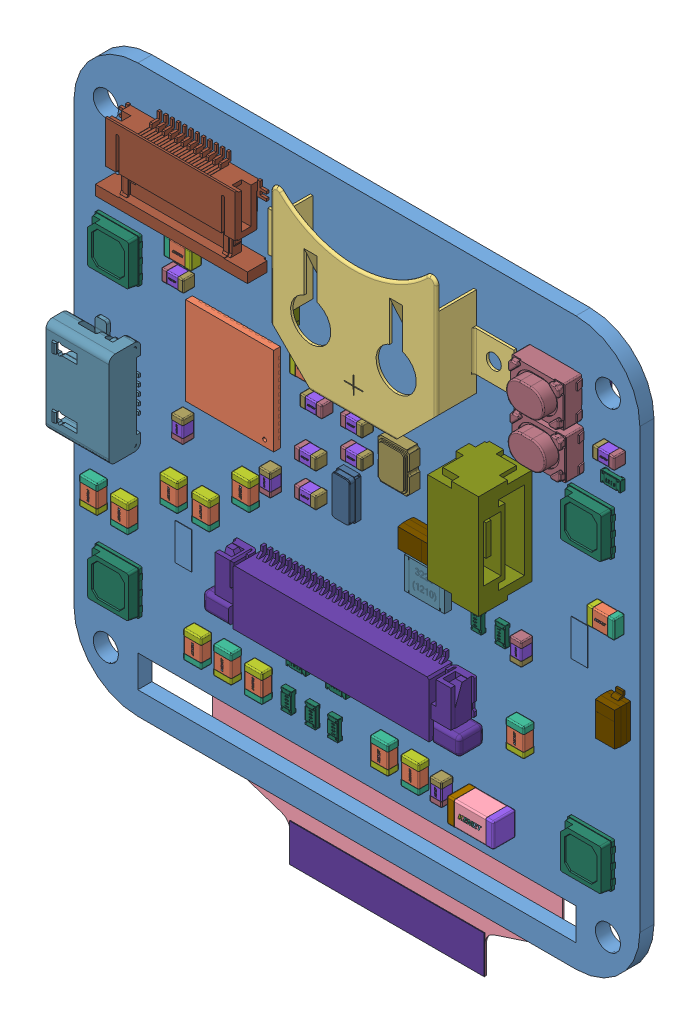
SolidWorks assembly PCB_2020-12-27_16-28-50_2021-02-20_20-59-34, configuration 默认. Lengths in mm.
Overall size (45.01 51.47 7.58).
307 component instances, 72 part files, 0 mates.
Components (placement in the parent):
- PCB_2020-12-27_16-28-50_2021-02-20_20-59-34.step-1: PCB_2020-12-27_16-28-50_2021-02-20_20-59-34.step [默认] at origin size (45.01 51.47 7.58)
  - Board.step-1: Board.step [默认] at origin size (45.01 45.01 1.12)
    - Open CASCADE STEP translator 6.8 3.1.1.step-1: Open CASCADE STEP translator 6.8 3.1.1.step [默认] at (0 0 -1.1227) size (45.01 45.01 1.12)
  - C34.step-1: C34.step [默认] at origin size (2.2 1.45 0.88)
    - c0805c101k5gactu.step-1: c0805c101k5gactu.step [默认] at (159.963 120.323 -10.6426) x (1 0 0) z (0 -1 0) size (2.2 0.88 1.45)
      - Open CASCADE STEP translator 6.8 3.2.1.1.step-1: Open CASCADE STEP translator 6.8 3.2.1.1.step [默认] at origin size (2 0.86 1.43)
      - Open CASCADE STEP translator 6.8 3.2.1.2.step-1: Open CASCADE STEP translator 6.8 3.2.1.2.step [默认] at origin size (0.34 0 0.18)
      - Open CASCADE STEP translator 6.8 3.2.1.3.step-1: Open CASCADE STEP translator 6.8 3.2.1.3.step [默认] at origin size (0.41 0 0.18)
      - Open CASCADE STEP translator 6.8 3.2.1.4.step-1: Open CASCADE STEP translator 6.8 3.2.1.4.step [默认] at origin size (0.21 0 0.18)
      - Open CASCADE STEP translator 6.8 3.2.1.5.step-1: Open CASCADE STEP translator 6.8 3.2.1.5.step [默认] at origin size (0.5 0.88 1.45)
      - Open CASCADE STEP translator 6.8 3.2.1.6.step-1: Open CASCADE STEP translator 6.8 3.2.1.6.step [默认] at origin size (0.5 0.88 1.45)
  - C14.step-1: C14.step [默认] at origin size (1.45 2.2 0.88)
    - c0805c101k5gactu.step-1: c0805c101k5gactu.step [默认] at (101.7169 -30.907 -10.6426) x (0 -1 0) z (-1 0 0) size (2.2 0.88 1.45)
      - Open CASCADE STEP translator 6.8 3.2.1.1.step-1: Open CASCADE STEP translator 6.8 3.2.1.1.step [默认] at origin size (2 0.86 1.43)
      - Open CASCADE STEP translator 6.8 3.2.1.2.step-1: Open CASCADE STEP translator 6.8 3.2.1.2.step [默认] at origin size (0.34 0 0.18)
      - Open CASCADE STEP translator 6.8 3.2.1.3.step-1: Open CASCADE STEP translator 6.8 3.2.1.3.step [默认] at origin size (0.41 0 0.18)
      - Open CASCADE STEP translator 6.8 3.2.1.4.step-1: Open CASCADE STEP translator 6.8 3.2.1.4.step [默认] at origin size (0.21 0 0.18)
      - Open CASCADE STEP translator 6.8 3.2.1.5.step-1: Open CASCADE STEP translator 6.8 3.2.1.5.step [默认] at origin size (0.5 0.88 1.45)
      - Open CASCADE STEP translator 6.8 3.2.1.6.step-1: Open CASCADE STEP translator 6.8 3.2.1.6.step [默认] at origin size (0.5 0.88 1.45)
  - C13.step-1: C13.step [默认] at origin size (0.95 1.77 0.95)
    - c0603x104k3ractu.step-1: c0603x104k3ractu.step [默认] at (16.3625 164.212 -10.6426) x (0 1 0) z (1 0 0) size (1.77 0.95 0.95)
      - Open CASCADE STEP translator 6.8 3.4.1.1.step-1: Open CASCADE STEP translator 6.8 3.4.1.1.step [默认] at origin size (1.57 0.93 0.93)
      - Open CASCADE STEP translator 6.8 3.4.1.2.step-1: Open CASCADE STEP translator 6.8 3.4.1.2.step [默认] at origin size (0.24 0 0.13)
      - Open CASCADE STEP translator 6.8 3.4.1.3.step-1: Open CASCADE STEP translator 6.8 3.4.1.3.step [默认] at origin size (0.29 0 0.13)
      - Open CASCADE STEP translator 6.8 3.4.1.4.step-1: Open CASCADE STEP translator 6.8 3.4.1.4.step [默认] at origin size (0.15 0 0.13)
      - Open CASCADE STEP translator 6.8 3.4.1.5.step-1: Open CASCADE STEP translator 6.8 3.4.1.5.step [默认] at origin size (0.45 0.95 0.95)
      - Open CASCADE STEP translator 6.8 3.4.1.6.step-1: Open CASCADE STEP translator 6.8 3.4.1.6.step [默认] at origin size (0.45 0.95 0.95)
  - C12.step-1: C12.step [默认] at origin size (0.95 1.77 0.95)
    - c0603x104k3ractu.step-1: c0603x104k3ractu.step [默认] at (9.3976 164.422 -10.6426) x (0 1 0) z (1 0 0) size (1.77 0.95 0.95)
      - Open CASCADE STEP translator 6.8 3.4.1.1.step-1: Open CASCADE STEP translator 6.8 3.4.1.1.step [默认] at origin size (1.57 0.93 0.93)
      - Open CASCADE STEP translator 6.8 3.4.1.2.step-1: Open CASCADE STEP translator 6.8 3.4.1.2.step [默认] at origin size (0.24 0 0.13)
      - Open CASCADE STEP translator 6.8 3.4.1.3.step-1: Open CASCADE STEP translator 6.8 3.4.1.3.step [默认] at origin size (0.29 0 0.13)
      - Open CASCADE STEP translator 6.8 3.4.1.4.step-1: Open CASCADE STEP translator 6.8 3.4.1.4.step [默认] at origin size (0.15 0 0.13)
      - Open CASCADE STEP translator 6.8 3.4.1.5.step-1: Open CASCADE STEP translator 6.8 3.4.1.5.step [默认] at origin size (0.45 0.95 0.95)
      - Open CASCADE STEP translator 6.8 3.4.1.6.step-1: Open CASCADE STEP translator 6.8 3.4.1.6.step [默认] at origin size (0.45 0.95 0.95)
  - USB2.step-1: USB2.step [默认] at origin size (5 7.8 2.7)
    - User_Library-micro_usb_SMD_RGB8421504.step-1: User_Library-micro_usb_SMD_RGB8421504.step [默认] at (44.3599 67.8551 1.27) x (0 -1 0) z (-1 0 0) size (7.8 2.7 5)
  - R7.step-1: R7.step [默认] at origin size (1.6 0.8 0.42)
    - User_Library-Res-0603.step-1: User_Library-Res-0603.step [默认] at (87.122 80.8989 0) x (-1 0 0) z (0 1 0) size (1.6 0.42 0.8)
  - L2.step-1: L2.step [默认] at origin size (0.86 1.6 0.51)
    - CircuitWorks-RESISTOR_0603.step-1: CircuitWorks-RESISTOR_0603.step [默认] at (61.595 79.7559 0) x (0 -1 0) z (-1 0 0) size (1.6 0.51 0.86)
  - P2.step-1: P2.step [默认] at origin size (20.43 5.11 2.05)
    - 3-1734839-0_RGB8421504.step-1: 3-1734839-0_RGB8421504.step [默认] at (66.548 57.4041 1.0414) x (1 0 0) z (0 -1 0) size (20.43 2.05 5.11)
  - D4.step-1: D4.step [默认] at origin size (3.7 1.6 1.27)
    - CircuitWorks-SOD123.step-1: CircuitWorks-SOD123.step [默认] at (72.4968 69.5129 0.0508) x (1 0 0) z (0 -1 0) size (3.7 1.27 1.6)
  - D5.step-1: D5.step [默认] at origin size (1.6 3.7 1.27)
    - CircuitWorks-SOD123.step-1: CircuitWorks-SOD123.step [默认] at (87.6301 64.8969 0.0508) x (0 1 0) z (1 0 0) size (3.7 1.27 1.6)
  - C21.step-1: C21.step [默认] at origin size (1.45 2.2 0.88)
    - c0805c101k5gactu.step-1: c0805c101k5gactu.step [默认] at (98.5419 -33.828 -10.6426) x (0 -1 0) z (-1 0 0) size (2.2 0.88 1.45)
      - Open CASCADE STEP translator 6.8 3.2.1.1.step-1: Open CASCADE STEP translator 6.8 3.2.1.1.step [默认] at origin size (2 0.86 1.43)
      - Open CASCADE STEP translator 6.8 3.2.1.2.step-1: Open CASCADE STEP translator 6.8 3.2.1.2.step [默认] at origin size (0.34 0 0.18)
      - Open CASCADE STEP translator 6.8 3.2.1.3.step-1: Open CASCADE STEP translator 6.8 3.2.1.3.step [默认] at origin size (0.41 0 0.18)
      - Open CASCADE STEP translator 6.8 3.2.1.4.step-1: Open CASCADE STEP translator 6.8 3.2.1.4.step [默认] at origin size (0.21 0 0.18)
      - Open CASCADE STEP translator 6.8 3.2.1.5.step-1: Open CASCADE STEP translator 6.8 3.2.1.5.step [默认] at origin size (0.5 0.88 1.45)
      - Open CASCADE STEP translator 6.8 3.2.1.6.step-1: Open CASCADE STEP translator 6.8 3.2.1.6.step [默认] at origin size (0.5 0.88 1.45)
  - C24.step-1: C24.step [默认] at origin size (1.45 2.2 0.88)
    - c0805c101k5gactu.step-1: c0805c101k5gactu.step [默认] at (2.51 156.471 -10.6426) x (0 1 0) z (1 0 0) size (2.2 0.88 1.45)
      - Open CASCADE STEP translator 6.8 3.2.1.1.step-1: Open CASCADE STEP translator 6.8 3.2.1.1.step [默认] at origin size (2 0.86 1.43)
      - Open CASCADE STEP translator 6.8 3.2.1.2.step-1: Open CASCADE STEP translator 6.8 3.2.1.2.step [默认] at origin size (0.34 0 0.18)
      - Open CASCADE STEP translator 6.8 3.2.1.3.step-1: Open CASCADE STEP translator 6.8 3.2.1.3.step [默认] at origin size (0.41 0 0.18)
      - Open CASCADE STEP translator 6.8 3.2.1.4.step-1: Open CASCADE STEP translator 6.8 3.2.1.4.step [默认] at origin size (0.21 0 0.18)
      - Open CASCADE STEP translator 6.8 3.2.1.5.step-1: Open CASCADE STEP translator 6.8 3.2.1.5.step [默认] at origin size (0.5 0.88 1.45)
      - Open CASCADE STEP translator 6.8 3.2.1.6.step-1: Open CASCADE STEP translator 6.8 3.2.1.6.step [默认] at origin size (0.5 0.88 1.45)
  - U7.step-1: U7.step [默认] at origin size (2.5 3 1.1)
    - CircuitWorks-SOT-23-5.step-1: CircuitWorks-SOT-23-5.step [默认] at (84.308 68.2431 -0.5131) x (0 1 0) z (1 0 0) size (3 1.1 2.5)
  - U5.step-1: U5.step [默认] at origin size (7 7 0.55)
    - User_Library-UFQFPN48.step-1: User_Library-UFQFPN48.step [默认] at (57.0029 73.1959 0) x (-1 0 0) z (0 0 1) size (7 7 0.55)
  - R13.step-1: R13.step [默认] at origin size (0.8 1.6 0.42)
    - User_Library-Res-0603.step-1: User_Library-Res-0603.step [默认] at (78.3388 65.957 0) x (0 1 0) z (1 0 0) size (1.6 0.42 0.8)
  - U4.step-1: U4.step [默认] at origin size (19.57 12.72 3.54)
    - User_Library-BK-885-TR.step-1: User_Library-BK-885-TR.step [默认] at (69.4691 84.328 0) x (1 0 0) z (0 -1 0) size (19.57 3.54 12.72)
  - U3.step-1: U3.step [默认] at origin size (0.8 1.6 0.42)
    - User_Library-Res-0603.step-1: User_Library-Res-0603.step [默认] at (61.3211 52.876 0) x (0 -1 0) z (-1 0 0) size (1.6 0.42 0.8)
  - C27.step-1: C27.step [默认] at origin size (0.95 1.77 0.95)
    - c0603x104k3ractu.step-1: c0603x104k3ractu.step [默认] at (123.9324 -30.647 -10.6426) x (0 -1 0) z (-1 0 0) size (1.77 0.95 0.95)
      - Open CASCADE STEP translator 6.8 3.4.1.1.step-1: Open CASCADE STEP translator 6.8 3.4.1.1.step [默认] at origin size (1.57 0.93 0.93)
      - Open CASCADE STEP translator 6.8 3.4.1.2.step-1: Open CASCADE STEP translator 6.8 3.4.1.2.step [默认] at origin size (0.24 0 0.13)
      - Open CASCADE STEP translator 6.8 3.4.1.3.step-1: Open CASCADE STEP translator 6.8 3.4.1.3.step [默认] at origin size (0.29 0 0.13)
      - Open CASCADE STEP translator 6.8 3.4.1.4.step-1: Open CASCADE STEP translator 6.8 3.4.1.4.step [默认] at origin size (0.15 0 0.13)
      - Open CASCADE STEP translator 6.8 3.4.1.5.step-1: Open CASCADE STEP translator 6.8 3.4.1.5.step [默认] at origin size (0.45 0.95 0.95)
      - Open CASCADE STEP translator 6.8 3.4.1.6.step-1: Open CASCADE STEP translator 6.8 3.4.1.6.step [默认] at origin size (0.45 0.95 0.95)
  - C20.step-1: C20.step [默认] at origin size (3.7 1.95 1.8)
    - c1206x223j2gacauto.step-1: c1206x223j2gacauto.step [默认] at (174.9253 96.5054 -10.6426) x (1 0 0) z (0 -1 0) size (3.7 1.8 1.95)
      - Open CASCADE STEP translator 6.8 3.20.1.1.step-1: Open CASCADE STEP translator 6.8 3.20.1.1.step [默认] at origin size (3.5 1.78 1.93)
      - Open CASCADE STEP translator 6.8 3.20.1.2.step-1: Open CASCADE STEP translator 6.8 3.20.1.2.step [默认] at origin size (0.7 0 0.37)
      - Open CASCADE STEP translator 6.8 3.20.1.3.step-1: Open CASCADE STEP translator 6.8 3.20.1.3.step [默认] at origin size (0.85 0 0.37)
      - Open CASCADE STEP translator 6.8 3.20.1.4.step-1: Open CASCADE STEP translator 6.8 3.20.1.4.step [默认] at origin size (0.44 0 0.37)
      - Open CASCADE STEP translator 6.8 3.20.1.5.step-1: Open CASCADE STEP translator 6.8 3.20.1.5.step [默认] at origin size (0.6 1.8 1.95)
      - Open CASCADE STEP translator 6.8 3.20.1.6.step-1: Open CASCADE STEP translator 6.8 3.20.1.6.step [默认] at origin size (0.6 1.8 1.95)
  - X3.step-1: X3.step [默认] at origin size (1.5 3.2 0.91)
    - crystal_rtf3215.step-1: crystal_rtf3215.step [默认] at (66.167 69.4691 0) x (0 1 0) z (1 0 0) size (3.2 0.91 1.5)
  - C28.step-1: C28.step [默认] at origin size (1.45 2.2 0.88)
    - c0805c101k5gactu.step-1: c0805c101k5gactu.step [默认] at (25.644 150.077 -10.6426) x (0 1 0) z (1 0 0) size (2.2 0.88 1.45)
      - Open CASCADE STEP translator 6.8 3.2.1.1.step-1: Open CASCADE STEP translator 6.8 3.2.1.1.step [默认] at origin size (2 0.86 1.43)
      - Open CASCADE STEP translator 6.8 3.2.1.2.step-1: Open CASCADE STEP translator 6.8 3.2.1.2.step [默认] at origin size (0.34 0 0.18)
      - Open CASCADE STEP translator 6.8 3.2.1.3.step-1: Open CASCADE STEP translator 6.8 3.2.1.3.step [默认] at origin size (0.41 0 0.18)
      - Open CASCADE STEP translator 6.8 3.2.1.4.step-1: Open CASCADE STEP translator 6.8 3.2.1.4.step [默认] at origin size (0.21 0 0.18)
      - Open CASCADE STEP translator 6.8 3.2.1.5.step-1: Open CASCADE STEP translator 6.8 3.2.1.5.step [默认] at origin size (0.5 0.88 1.45)
      - Open CASCADE STEP translator 6.8 3.2.1.6.step-1: Open CASCADE STEP translator 6.8 3.2.1.6.step [默认] at origin size (0.5 0.88 1.45)
  - C29.step-1: C29.step [默认] at origin size (1.45 2.2 0.88)
    - c0805c101k5gactu.step-1: c0805c101k5gactu.step [默认] at (102.7329 -43.6071 -10.6426) x (0 -1 0) z (-1 0 0) size (2.2 0.88 1.45)
      - Open CASCADE STEP translator 6.8 3.2.1.1.step-1: Open CASCADE STEP translator 6.8 3.2.1.1.step [默认] at origin size (2 0.86 1.43)
      - Open CASCADE STEP translator 6.8 3.2.1.2.step-1: Open CASCADE STEP translator 6.8 3.2.1.2.step [默认] at origin size (0.34 0 0.18)
      - Open CASCADE STEP translator 6.8 3.2.1.3.step-1: Open CASCADE STEP translator 6.8 3.2.1.3.step [默认] at origin size (0.41 0 0.18)
      - Open CASCADE STEP translator 6.8 3.2.1.4.step-1: Open CASCADE STEP translator 6.8 3.2.1.4.step [默认] at origin size (0.21 0 0.18)
      - Open CASCADE STEP translator 6.8 3.2.1.5.step-1: Open CASCADE STEP translator 6.8 3.2.1.5.step [默认] at origin size (0.5 0.88 1.45)
      - Open CASCADE STEP translator 6.8 3.2.1.6.step-1: Open CASCADE STEP translator 6.8 3.2.1.6.step [默认] at origin size (0.5 0.88 1.45)
  - C30.step-1: C30.step [默认] at origin size (1.45 2.2 0.88)
    - c0805c101k5gactu.step-1: c0805c101k5gactu.step [默认] at (97.9069 -43.6071 -10.6426) x (0 -1 0) z (-1 0 0) size (2.2 0.88 1.45)
      - Open CASCADE STEP translator 6.8 3.2.1.1.step-1: Open CASCADE STEP translator 6.8 3.2.1.1.step [默认] at origin size (2 0.86 1.43)
      - Open CASCADE STEP translator 6.8 3.2.1.2.step-1: Open CASCADE STEP translator 6.8 3.2.1.2.step [默认] at origin size (0.34 0 0.18)
      - Open CASCADE STEP translator 6.8 3.2.1.3.step-1: Open CASCADE STEP translator 6.8 3.2.1.3.step [默认] at origin size (0.41 0 0.18)
      - Open CASCADE STEP translator 6.8 3.2.1.4.step-1: Open CASCADE STEP translator 6.8 3.2.1.4.step [默认] at origin size (0.21 0 0.18)
      - Open CASCADE STEP translator 6.8 3.2.1.5.step-1: Open CASCADE STEP translator 6.8 3.2.1.5.step [默认] at origin size (0.5 0.88 1.45)
      - Open CASCADE STEP translator 6.8 3.2.1.6.step-1: Open CASCADE STEP translator 6.8 3.2.1.6.step [默认] at origin size (0.5 0.88 1.45)
  - U6.step-1: U6.step [默认] at origin size (2.5 3 1.1)
    - CircuitWorks-SOT-23-5.step-1: CircuitWorks-SOT-23-5.step [默认] at (52.8119 59.0989 -0.5131) x (0 -1 0) z (-1 0 0) size (3 1.1 2.5)
  - FPC1.step-1: FPC1.step [默认] at origin size (12.1 6.6 2)
    - 52746-1290_RGB10066329.step-1: 52746-1290_RGB10066329.step [默认] at (53.7211 87.5031 0) x (1 0 0) z (0 -1 0) size (12.1 2 6.6)
  - C18.step-1: C18.step [默认] at origin size (0.95 1.77 0.95)
    - c0603x104k3ractu.step-1: c0603x104k3ractu.step [默认] at (29.9716 149.69 -10.6426) x (0 1 0) z (1 0 0) size (1.77 0.95 0.95)
      - Open CASCADE STEP translator 6.8 3.4.1.1.step-1: Open CASCADE STEP translator 6.8 3.4.1.1.step [默认] at origin size (1.57 0.93 0.93)
      - Open CASCADE STEP translator 6.8 3.4.1.2.step-1: Open CASCADE STEP translator 6.8 3.4.1.2.step [默认] at origin size (0.24 0 0.13)
      - Open CASCADE STEP translator 6.8 3.4.1.3.step-1: Open CASCADE STEP translator 6.8 3.4.1.3.step [默认] at origin size (0.29 0 0.13)
      - Open CASCADE STEP translator 6.8 3.4.1.4.step-1: Open CASCADE STEP translator 6.8 3.4.1.4.step [默认] at origin size (0.15 0 0.13)
      - Open CASCADE STEP translator 6.8 3.4.1.5.step-1: Open CASCADE STEP translator 6.8 3.4.1.5.step [默认] at origin size (0.45 0.95 0.95)
      - Open CASCADE STEP translator 6.8 3.4.1.6.step-1: Open CASCADE STEP translator 6.8 3.4.1.6.step [默认] at origin size (0.45 0.95 0.95)
  - X1.step-1: X1.step [默认] at origin size (2.5 3.2 1.05)
    - User_Library-SMD-3225_4P.step-1: User_Library-SMD-3225_4P.step [默认] at (70.338 73.8309 0) x (0 -1 0) z (0 0 1) size (3.2 2.5 1.05)
  - C26.step-1: C26.step [默认] at origin size (2.2 1.45 0.88)
    - c0805c101k5gactu.step-1: c0805c101k5gactu.step [默认] at (183.605 114.818 -10.6426) x (1 0 0) z (0 -1 0) size (2.2 0.88 1.45)
      - Open CASCADE STEP translator 6.8 3.2.1.1.step-1: Open CASCADE STEP translator 6.8 3.2.1.1.step [默认] at origin size (2 0.86 1.43)
      - Open CASCADE STEP translator 6.8 3.2.1.2.step-1: Open CASCADE STEP translator 6.8 3.2.1.2.step [默认] at origin size (0.34 0 0.18)
      - Open CASCADE STEP translator 6.8 3.2.1.3.step-1: Open CASCADE STEP translator 6.8 3.2.1.3.step [默认] at origin size (0.41 0 0.18)
      - Open CASCADE STEP translator 6.8 3.2.1.4.step-1: Open CASCADE STEP translator 6.8 3.2.1.4.step [默认] at origin size (0.21 0 0.18)
      - Open CASCADE STEP translator 6.8 3.2.1.5.step-1: Open CASCADE STEP translator 6.8 3.2.1.5.step [默认] at origin size (0.5 0.88 1.45)
      - Open CASCADE STEP translator 6.8 3.2.1.6.step-1: Open CASCADE STEP translator 6.8 3.2.1.6.step [默认] at origin size (0.5 0.88 1.45)
  - C25.step-1: C25.step [默认] at origin size (1.45 2.2 0.88)
    - c0805c101k5gactu.step-1: c0805c101k5gactu.step [默认] at (36.439 156.681 -10.6426) x (0 1 0) z (1 0 0) size (2.2 0.88 1.45)
      - Open CASCADE STEP translator 6.8 3.2.1.1.step-1: Open CASCADE STEP translator 6.8 3.2.1.1.step [默认] at origin size (2 0.86 1.43)
      - Open CASCADE STEP translator 6.8 3.2.1.2.step-1: Open CASCADE STEP translator 6.8 3.2.1.2.step [默认] at origin size (0.34 0 0.18)
      - Open CASCADE STEP translator 6.8 3.2.1.3.step-1: Open CASCADE STEP translator 6.8 3.2.1.3.step [默认] at origin size (0.41 0 0.18)
      - Open CASCADE STEP translator 6.8 3.2.1.4.step-1: Open CASCADE STEP translator 6.8 3.2.1.4.step [默认] at origin size (0.21 0 0.18)
      - Open CASCADE STEP translator 6.8 3.2.1.5.step-1: Open CASCADE STEP translator 6.8 3.2.1.5.step [默认] at origin size (0.5 0.88 1.45)
      - Open CASCADE STEP translator 6.8 3.2.1.6.step-1: Open CASCADE STEP translator 6.8 3.2.1.6.step [默认] at origin size (0.5 0.88 1.45)
  - R17.step-1: R17.step [默认] at origin size (1.6 0.8 0.42)
    - User_Library-Res-0603.step-1: User_Library-Res-0603.step [默认] at (65.278 55.7531 0) x (1 0 0) z (0 -1 0) size (1.6 0.42 0.8)
  - R12.step-1: R12.step [默认] at origin size (0.8 1.6 0.42)
    - User_Library-Res-0603.step-1: User_Library-Res-0603.step [默认] at (63.2461 52.832 0) x (0 -1 0) z (-1 0 0) size (1.6 0.42 0.8)
  - R16.step-1: R16.step [默认] at origin size (1.6 0.8 0.42)
    - User_Library-Res-0603.step-1: User_Library-Res-0603.step [默认] at (62.103 55.7529 0) x (-1 0 0) z (0 1 0) size (1.6 0.42 0.8)
  - R15.step-1: R15.step [默认] at origin size (0.8 1.6 0.42)
    - User_Library-Res-0603.step-1: User_Library-Res-0603.step [默认] at (65.0241 52.832 0) x (0 -1 0) z (-1 0 0) size (1.6 0.42 0.8)
  - SW2.step-1: SW2.step [默认] at origin size (4.6 3.2 2.5)
    - skrpace010_RGB10066329.step-1: skrpace010_RGB10066329.step [默认] at (82.5499 81.661 0) x (-1 0 0) z (0 1 0) size (4.6 2.5 3.2)
  - SW1.step-1: SW1.step [默认] at origin size (4.6 3.2 2.5)
    - skrpace010_RGB10066329.step-1: skrpace010_RGB10066329.step [默认] at (82.4231 85.217 0) x (1 0 0) z (0 -1 0) size (4.6 2.5 3.2)
  - C17.step-1: C17.step [默认] at origin size (1.77 0.95 0.95)
    - c0603x104k3ractu.step-1: c0603x104k3ractu.step [默认] at (159.977 114.6814 -10.6426) x (1 0 0) z (0 -1 0) size (1.77 0.95 0.95)
      - Open CASCADE STEP translator 6.8 3.4.1.1.step-1: Open CASCADE STEP translator 6.8 3.4.1.1.step [默认] at origin size (1.57 0.93 0.93)
      - Open CASCADE STEP translator 6.8 3.4.1.2.step-1: Open CASCADE STEP translator 6.8 3.4.1.2.step [默认] at origin size (0.24 0 0.13)
      - Open CASCADE STEP translator 6.8 3.4.1.3.step-1: Open CASCADE STEP translator 6.8 3.4.1.3.step [默认] at origin size (0.29 0 0.13)
      - Open CASCADE STEP translator 6.8 3.4.1.4.step-1: Open CASCADE STEP translator 6.8 3.4.1.4.step [默认] at origin size (0.15 0 0.13)
      - Open CASCADE STEP translator 6.8 3.4.1.5.step-1: Open CASCADE STEP translator 6.8 3.4.1.5.step [默认] at origin size (0.45 0.95 0.95)
      - Open CASCADE STEP translator 6.8 3.4.1.6.step-1: Open CASCADE STEP translator 6.8 3.4.1.6.step [默认] at origin size (0.45 0.95 0.95)
  - C19.step-1: C19.step [默认] at origin size (1.77 0.95 0.95)
    - c0603x104k3ractu.step-1: c0603x104k3ractu.step [默认] at (159.977 112.0144 -10.6426) x (1 0 0) z (0 -1 0) size (1.77 0.95 0.95)
      - Open CASCADE STEP translator 6.8 3.4.1.1.step-1: Open CASCADE STEP translator 6.8 3.4.1.1.step [默认] at origin size (1.57 0.93 0.93)
      - Open CASCADE STEP translator 6.8 3.4.1.2.step-1: Open CASCADE STEP translator 6.8 3.4.1.2.step [默认] at origin size (0.24 0 0.13)
      - Open CASCADE STEP translator 6.8 3.4.1.3.step-1: Open CASCADE STEP translator 6.8 3.4.1.3.step [默认] at origin size (0.29 0 0.13)
      - Open CASCADE STEP translator 6.8 3.4.1.4.step-1: Open CASCADE STEP translator 6.8 3.4.1.4.step [默认] at origin size (0.15 0 0.13)
      - Open CASCADE STEP translator 6.8 3.4.1.5.step-1: Open CASCADE STEP translator 6.8 3.4.1.5.step [默认] at origin size (0.45 0.95 0.95)
      - Open CASCADE STEP translator 6.8 3.4.1.6.step-1: Open CASCADE STEP translator 6.8 3.4.1.6.step [默认] at origin size (0.45 0.95 0.95)
  - C16.step-1: C16.step [默认] at origin size (1.77 0.95 0.95)
    - c0603x104k3ractu.step-1: c0603x104k3ractu.step [默认] at (163.64 118.7894 -10.6426) x (1 0 0) z (0 -1 0) size (1.77 0.95 0.95)
      - Open CASCADE STEP translator 6.8 3.4.1.1.step-1: Open CASCADE STEP translator 6.8 3.4.1.1.step [默认] at origin size (1.57 0.93 0.93)
      - Open CASCADE STEP translator 6.8 3.4.1.2.step-1: Open CASCADE STEP translator 6.8 3.4.1.2.step [默认] at origin size (0.24 0 0.13)
      - Open CASCADE STEP translator 6.8 3.4.1.3.step-1: Open CASCADE STEP translator 6.8 3.4.1.3.step [默认] at origin size (0.29 0 0.13)
      - Open CASCADE STEP translator 6.8 3.4.1.4.step-1: Open CASCADE STEP translator 6.8 3.4.1.4.step [默认] at origin size (0.15 0 0.13)
      - Open CASCADE STEP translator 6.8 3.4.1.5.step-1: Open CASCADE STEP translator 6.8 3.4.1.5.step [默认] at origin size (0.45 0.95 0.95)
      - Open CASCADE STEP translator 6.8 3.4.1.6.step-1: Open CASCADE STEP translator 6.8 3.4.1.6.step [默认] at origin size (0.45 0.95 0.95)
  - C15.step-1: C15.step [默认] at origin size (1.77 0.95 0.95)
    - c0603x104k3ractu.step-1: c0603x104k3ractu.step [默认] at (163.64 116.5034 -10.6426) x (1 0 0) z (0 -1 0) size (1.77 0.95 0.95)
      - Open CASCADE STEP translator 6.8 3.4.1.1.step-1: Open CASCADE STEP translator 6.8 3.4.1.1.step [默认] at origin size (1.57 0.93 0.93)
      - Open CASCADE STEP translator 6.8 3.4.1.2.step-1: Open CASCADE STEP translator 6.8 3.4.1.2.step [默认] at origin size (0.24 0 0.13)
      - Open CASCADE STEP translator 6.8 3.4.1.3.step-1: Open CASCADE STEP translator 6.8 3.4.1.3.step [默认] at origin size (0.29 0 0.13)
      - Open CASCADE STEP translator 6.8 3.4.1.4.step-1: Open CASCADE STEP translator 6.8 3.4.1.4.step [默认] at origin size (0.15 0 0.13)
      - Open CASCADE STEP translator 6.8 3.4.1.5.step-1: Open CASCADE STEP translator 6.8 3.4.1.5.step [默认] at origin size (0.45 0.95 0.95)
      - Open CASCADE STEP translator 6.8 3.4.1.6.step-1: Open CASCADE STEP translator 6.8 3.4.1.6.step [默认] at origin size (0.45 0.95 0.95)
  - R14.step-1: R14.step [默认] at origin size (0.8 1.6 0.42)
    - User_Library-Res-0603.step-1: User_Library-Res-0603.step [默认] at (76.4338 65.957 0) x (0 1 0) z (1 0 0) size (1.6 0.42 0.8)
  - R11.step-1: R11.step [默认] at origin size (3.2 2.51 0.55)
    - User_Library-RESC3225X06N.step-1: User_Library-RESC3225X06N.step [默认] at (72.4971 66.592 0) size (3.2 2.51 0.55)
  - C23.step-1: C23.step [默认] at origin size (1.45 2.2 0.88)
    - c0805c101k5gactu.step-1: c0805c101k5gactu.step [默认] at (92.0649 -37.257 -10.6426) x (0 -1 0) z (-1 0 0) size (2.2 0.88 1.45)
      - Open CASCADE STEP translator 6.8 3.2.1.1.step-1: Open CASCADE STEP translator 6.8 3.2.1.1.step [默认] at origin size (2 0.86 1.43)
      - Open CASCADE STEP translator 6.8 3.2.1.2.step-1: Open CASCADE STEP translator 6.8 3.2.1.2.step [默认] at origin size (0.34 0 0.18)
      - Open CASCADE STEP translator 6.8 3.2.1.3.step-1: Open CASCADE STEP translator 6.8 3.2.1.3.step [默认] at origin size (0.41 0 0.18)
      - Open CASCADE STEP translator 6.8 3.2.1.4.step-1: Open CASCADE STEP translator 6.8 3.2.1.4.step [默认] at origin size (0.21 0 0.18)
      - Open CASCADE STEP translator 6.8 3.2.1.5.step-1: Open CASCADE STEP translator 6.8 3.2.1.5.step [默认] at origin size (0.5 0.88 1.45)
      - Open CASCADE STEP translator 6.8 3.2.1.6.step-1: Open CASCADE STEP translator 6.8 3.2.1.6.step [默认] at origin size (0.5 0.88 1.45)
  - C22.step-1: C22.step [默认] at origin size (1.45 2.2 0.88)
    - c0805c101k5gactu.step-1: c0805c101k5gactu.step [默认] at (96.0019 -33.828 -10.6426) x (0 -1 0) z (-1 0 0) size (2.2 0.88 1.45)
      - Open CASCADE STEP translator 6.8 3.2.1.1.step-1: Open CASCADE STEP translator 6.8 3.2.1.1.step [默认] at origin size (2 0.86 1.43)
      - Open CASCADE STEP translator 6.8 3.2.1.2.step-1: Open CASCADE STEP translator 6.8 3.2.1.2.step [默认] at origin size (0.34 0 0.18)
      - Open CASCADE STEP translator 6.8 3.2.1.3.step-1: Open CASCADE STEP translator 6.8 3.2.1.3.step [默认] at origin size (0.41 0 0.18)
      - Open CASCADE STEP translator 6.8 3.2.1.4.step-1: Open CASCADE STEP translator 6.8 3.2.1.4.step [默认] at origin size (0.21 0 0.18)
      - Open CASCADE STEP translator 6.8 3.2.1.5.step-1: Open CASCADE STEP translator 6.8 3.2.1.5.step [默认] at origin size (0.5 0.88 1.45)
      - Open CASCADE STEP translator 6.8 3.2.1.6.step-1: Open CASCADE STEP translator 6.8 3.2.1.6.step [默认] at origin size (0.5 0.88 1.45)
  - LED2.step-1: LED2.step [默认] at origin size (3.6 3.5 0.95)
    - User_Library-WS2813_3535.step-1: User_Library-WS2813_3535.step [默认] at (47.732 54.273 0) x (1 0 0) z (0 -1 0) size (3.6 0.95 3.5)
  - LED3.step-1: LED3.step [默认] at origin size (3.6 3.5 0.95)
    - User_Library-WS2813_3535.step-1: User_Library-WS2813_3535.step [默认] at (47.732 77.133 0) x (1 0 0) z (0 -1 0) size (3.6 0.95 3.5)
  - LED5.step-1: LED5.step [默认] at origin size (3.6 3.5 0.95)
    - User_Library-WS2813_3535.step-1: User_Library-WS2813_3535.step [默认] at (85.324 54.273 0) x (1 0 0) z (0 -1 0) size (3.6 0.95 3.5)
  - LED4.step-1: LED4.step [默认] at origin size (3.6 3.5 0.95)
    - User_Library-WS2813_3535.step-1: User_Library-WS2813_3535.step [默认] at (85.324 77.133 0) x (1 0 0) z (0 -1 0) size (3.6 0.95 3.5)
  - C31.step-1: C31.step [默认] at origin size (1.45 2.2 0.88)
    - c0805c101k5gactu.step-1: c0805c101k5gactu.step [默认] at (115.199 -43.651 -10.6426) x (0 -1 0) z (-1 0 0) size (2.2 0.88 1.45)
      - Open CASCADE STEP translator 6.8 3.2.1.1.step-1: Open CASCADE STEP translator 6.8 3.2.1.1.step [默认] at origin size (2 0.86 1.43)
      - Open CASCADE STEP translator 6.8 3.2.1.2.step-1: Open CASCADE STEP translator 6.8 3.2.1.2.step [默认] at origin size (0.34 0 0.18)
      - Open CASCADE STEP translator 6.8 3.2.1.3.step-1: Open CASCADE STEP translator 6.8 3.2.1.3.step [默认] at origin size (0.41 0 0.18)
      - Open CASCADE STEP translator 6.8 3.2.1.4.step-1: Open CASCADE STEP translator 6.8 3.2.1.4.step [默认] at origin size (0.21 0 0.18)
      - Open CASCADE STEP translator 6.8 3.2.1.5.step-1: Open CASCADE STEP translator 6.8 3.2.1.5.step [默认] at origin size (0.5 0.88 1.45)
      - Open CASCADE STEP translator 6.8 3.2.1.6.step-1: Open CASCADE STEP translator 6.8 3.2.1.6.step [默认] at origin size (0.5 0.88 1.45)
  - C32.step-1: C32.step [默认] at origin size (1.45 2.2 0.88)
    - c0805c101k5gactu.step-1: c0805c101k5gactu.step [默认] at (13.178 150.121 -10.6426) x (0 1 0) z (1 0 0) size (2.2 0.88 1.45)
      - Open CASCADE STEP translator 6.8 3.2.1.1.step-1: Open CASCADE STEP translator 6.8 3.2.1.1.step [默认] at origin size (2 0.86 1.43)
      - Open CASCADE STEP translator 6.8 3.2.1.2.step-1: Open CASCADE STEP translator 6.8 3.2.1.2.step [默认] at origin size (0.34 0 0.18)
      - Open CASCADE STEP translator 6.8 3.2.1.3.step-1: Open CASCADE STEP translator 6.8 3.2.1.3.step [默认] at origin size (0.41 0 0.18)
      - Open CASCADE STEP translator 6.8 3.2.1.4.step-1: Open CASCADE STEP translator 6.8 3.2.1.4.step [默认] at origin size (0.21 0 0.18)
      - Open CASCADE STEP translator 6.8 3.2.1.5.step-1: Open CASCADE STEP translator 6.8 3.2.1.5.step [默认] at origin size (0.5 0.88 1.45)
      - Open CASCADE STEP translator 6.8 3.2.1.6.step-1: Open CASCADE STEP translator 6.8 3.2.1.6.step [默认] at origin size (0.5 0.88 1.45)
  - CN9.step-1: CN9.step [默认] at origin size (4.85 8.25 4.35)
    - User_Library-SM04B-GHS-TB_RGB14277081.step-1: User_Library-SM04B-GHS-TB_RGB14277081.step [默认] at (76.448 78.464 0) x (0 1 0) z (1 0 0) size (8.25 4.35 4.85)
  - C35.step-1: C35.step [默认] at origin size (1.77 0.95 0.95)
    - c0603x104k3ractu.step-1: c0603x104k3ractu.step [默认] at (-9.482 38.9886 -10.6426) x (-1 0 0) z (0 1 0) size (1.77 0.95 0.95)
      - Open CASCADE STEP translator 6.8 3.4.1.1.step-1: Open CASCADE STEP translator 6.8 3.4.1.1.step [默认] at origin size (1.57 0.93 0.93)
      - Open CASCADE STEP translator 6.8 3.4.1.2.step-1: Open CASCADE STEP translator 6.8 3.4.1.2.step [默认] at origin size (0.24 0 0.13)
      - Open CASCADE STEP translator 6.8 3.4.1.3.step-1: Open CASCADE STEP translator 6.8 3.4.1.3.step [默认] at origin size (0.29 0 0.13)
      - Open CASCADE STEP translator 6.8 3.4.1.4.step-1: Open CASCADE STEP translator 6.8 3.4.1.4.step [默认] at origin size (0.15 0 0.13)
      - Open CASCADE STEP translator 6.8 3.4.1.5.step-1: Open CASCADE STEP translator 6.8 3.4.1.5.step [默认] at origin size (0.45 0.95 0.95)
      - Open CASCADE STEP translator 6.8 3.4.1.6.step-1: Open CASCADE STEP translator 6.8 3.4.1.6.step [默认] at origin size (0.45 0.95 0.95)
  - C11.step-1: C11.step [默认] at origin size (1.77 0.95 0.95)
    - c0603x104k3ractu.step-1: c0603x104k3ractu.step [默认] at (149.436 121.6664 -10.6426) x (1 0 0) z (0 -1 0) size (1.77 0.95 0.95)
      - Open CASCADE STEP translator 6.8 3.4.1.1.step-1: Open CASCADE STEP translator 6.8 3.4.1.1.step [默认] at origin size (1.57 0.93 0.93)
      - Open CASCADE STEP translator 6.8 3.4.1.2.step-1: Open CASCADE STEP translator 6.8 3.4.1.2.step [默认] at origin size (0.24 0 0.13)
      - Open CASCADE STEP translator 6.8 3.4.1.3.step-1: Open CASCADE STEP translator 6.8 3.4.1.3.step [默认] at origin size (0.29 0 0.13)
      - Open CASCADE STEP translator 6.8 3.4.1.4.step-1: Open CASCADE STEP translator 6.8 3.4.1.4.step [默认] at origin size (0.15 0 0.13)
      - Open CASCADE STEP translator 6.8 3.4.1.5.step-1: Open CASCADE STEP translator 6.8 3.4.1.5.step [默认] at origin size (0.45 0.95 0.95)
      - Open CASCADE STEP translator 6.8 3.4.1.6.step-1: Open CASCADE STEP translator 6.8 3.4.1.6.step [默认] at origin size (0.45 0.95 0.95)
  - C36.step-1: C36.step [默认] at origin size (2.2 1.45 0.88)
    - c0805c101k5gactu.step-1: c0805c101k5gactu.step [默认] at (-43.651 36.312 -10.6426) x (-1 0 0) z (0 1 0) size (2.2 0.88 1.45)
      - Open CASCADE STEP translator 6.8 3.2.1.1.step-1: Open CASCADE STEP translator 6.8 3.2.1.1.step [默认] at origin size (2 0.86 1.43)
      - Open CASCADE STEP translator 6.8 3.2.1.2.step-1: Open CASCADE STEP translator 6.8 3.2.1.2.step [默认] at origin size (0.34 0 0.18)
      - Open CASCADE STEP translator 6.8 3.2.1.3.step-1: Open CASCADE STEP translator 6.8 3.2.1.3.step [默认] at origin size (0.41 0 0.18)
      - Open CASCADE STEP translator 6.8 3.2.1.4.step-1: Open CASCADE STEP translator 6.8 3.2.1.4.step [默认] at origin size (0.21 0 0.18)
      - Open CASCADE STEP translator 6.8 3.2.1.5.step-1: Open CASCADE STEP translator 6.8 3.2.1.5.step [默认] at origin size (0.5 0.88 1.45)
      - Open CASCADE STEP translator 6.8 3.2.1.6.step-1: Open CASCADE STEP translator 6.8 3.2.1.6.step [默认] at origin size (0.5 0.88 1.45)
  - C33.step-1: C33.step [默认] at origin size (1.77 0.95 0.95)
    - c0603x104k3ractu.step-1: c0603x104k3ractu.step [默认] at (-32.743 30.9046 -10.6426) x (-1 0 0) z (0 1 0) size (1.77 0.95 0.95)
      - Open CASCADE STEP translator 6.8 3.4.1.1.step-1: Open CASCADE STEP translator 6.8 3.4.1.1.step [默认] at origin size (1.57 0.93 0.93)
      - Open CASCADE STEP translator 6.8 3.4.1.2.step-1: Open CASCADE STEP translator 6.8 3.4.1.2.step [默认] at origin size (0.24 0 0.13)
      - Open CASCADE STEP translator 6.8 3.4.1.3.step-1: Open CASCADE STEP translator 6.8 3.4.1.3.step [默认] at origin size (0.29 0 0.13)
      - Open CASCADE STEP translator 6.8 3.4.1.4.step-1: Open CASCADE STEP translator 6.8 3.4.1.4.step [默认] at origin size (0.15 0 0.13)
      - Open CASCADE STEP translator 6.8 3.4.1.5.step-1: Open CASCADE STEP translator 6.8 3.4.1.5.step [默认] at origin size (0.45 0.95 0.95)
      - Open CASCADE STEP translator 6.8 3.4.1.6.step-1: Open CASCADE STEP translator 6.8 3.4.1.6.step [默认] at origin size (0.45 0.95 0.95)
  - Free-Models.step-1: Free-Models.step [默认] at origin size (33.8 46.35 1.8)
    - mcot128128az-rgbm.step-1: mcot128128az-rgbm.step [默认] at (83.7239 85.5761 -3.1293) x (-1 0 0) z (0 0 -1) size (33.8 46.35 1.8)
      - Open CASCADE STEP translator 6.8 3.56.1.1.step-1: Open CASCADE STEP translator 6.8 3.56.1.1.step [默认] at origin size (33.8 34 0.8)
      - Open CASCADE STEP translator 6.8 3.56.1.2.step-1: Open CASCADE STEP translator 6.8 3.56.1.2.step [默认] at origin size (33.8 32 0.8)
      - Open CASCADE STEP translator 6.8 3.56.1.3.step-1: Open CASCADE STEP translator 6.8 3.56.1.3.step [默认] at origin size (32.5 30.5 0.2)
      - Open CASCADE STEP translator 6.8 3.56.1.4.step-1: Open CASCADE STEP translator 6.8 3.56.1.4.step [默认] at origin size (28.86 28.86 0.1)
      - Open CASCADE STEP translator 6.8 3.56.1.5.step-1: Open CASCADE STEP translator 6.8 3.56.1.5.step [默认] at origin size (26.86 26.86 0.05)
      - Open CASCADE STEP translator 6.8 3.56.1.6.step-1: Open CASCADE STEP translator 6.8 3.56.1.6.step [默认] at origin size (27.83 14.35 0.12)
      - Open CASCADE STEP translator 6.8 3.56.1.7.step-1: Open CASCADE STEP translator 6.8 3.56.1.7.step [默认] at origin size (0.3 2 0.06)
      - Open CASCADE STEP translator 6.8 3.56.1.8.step-1: Open CASCADE STEP translator 6.8 3.56.1.8.step [默认] at origin size (0.3 2 0.06)
      - Open CASCADE STEP translator 6.8 3.56.1.9.step-1: Open CASCADE STEP translator 6.8 3.56.1.9.step [默认] at origin size (0.3 2 0.06)
      - Open CASCADE STEP translator 6.8 3.56.1.10.step-1: Open CASCADE STEP translator 6.8 3.56.1.10.step [默认] at origin size (0.3 2 0.06)
      - Open CASCADE STEP translator 6.8 3.56.1.11.step-1: Open CASCADE STEP translator 6.8 3.56.1.11.step [默认] at origin size (0.3 2 0.06)
      - Open CASCADE STEP translator 6.8 3.56.1.12.step-1: Open CASCADE STEP translator 6.8 3.56.1.12.step [默认] at origin size (0.3 2 0.06)
      - Open CASCADE STEP translator 6.8 3.56.1.13.step-1: Open CASCADE STEP translator 6.8 3.56.1.13.step [默认] at origin size (0.3 2 0.06)
      - Open CASCADE STEP translator 6.8 3.56.1.14.step-1: Open CASCADE STEP translator 6.8 3.56.1.14.step [默认] at origin size (0.3 2 0.06)
      - Open CASCADE STEP translator 6.8 3.56.1.15.step-1: Open CASCADE STEP translator 6.8 3.56.1.15.step [默认] at origin size (0.3 2 0.06)
      - Open CASCADE STEP translator 6.8 3.56.1.16.step-1: Open CASCADE STEP translator 6.8 3.56.1.16.step [默认] at origin size (0.3 2 0.06)
      - Open CASCADE STEP translator 6.8 3.56.1.17.step-1: Open CASCADE STEP translator 6.8 3.56.1.17.step [默认] at origin size (0.3 2 0.06)
      - Open CASCADE STEP translator 6.8 3.56.1.18.step-1: Open CASCADE STEP translator 6.8 3.56.1.18.step [默认] at origin size (0.3 2 0.06)
      - Open CASCADE STEP translator 6.8 3.56.1.19.step-1: Open CASCADE STEP translator 6.8 3.56.1.19.step [默认] at origin size (0.3 2 0.06)
      - Open CASCADE STEP translator 6.8 3.56.1.20.step-1: Open CASCADE STEP translator 6.8 3.56.1.20.step [默认] at origin size (0.3 2 0.06)
      - Open CASCADE STEP translator 6.8 3.56.1.21.step-1: Open CASCADE STEP translator 6.8 3.56.1.21.step [默认] at origin size (0.3 2 0.06)
      - Open CASCADE STEP translator 6.8 3.56.1.22.step-1: Open CASCADE STEP translator 6.8 3.56.1.22.step [默认] at origin size (0.3 2 0.06)
      - Open CASCADE STEP translator 6.8 3.56.1.23.step-1: Open CASCADE STEP translator 6.8 3.56.1.23.step [默认] at origin size (0.3 2 0.06)
      - Open CASCADE STEP translator 6.8 3.56.1.24.step-1: Open CASCADE STEP translator 6.8 3.56.1.24.step [默认] at origin size (0.3 2 0.06)
      - Open CASCADE STEP translator 6.8 3.56.1.25.step-1: Open CASCADE STEP translator 6.8 3.56.1.25.step [默认] at origin size (0.3 2 0.06)
      - Open CASCADE STEP translator 6.8 3.56.1.26.step-1: Open CASCADE STEP translator 6.8 3.56.1.26.step [默认] at origin size (0.3 2 0.06)
      - Open CASCADE STEP translator 6.8 3.56.1.27.step-1: Open CASCADE STEP translator 6.8 3.56.1.27.step [默认] at origin size (0.3 2 0.06)
      - Open CASCADE STEP translator 6.8 3.56.1.28.step-1: Open CASCADE STEP translator 6.8 3.56.1.28.step [默认] at origin size (0.3 2 0.06)
      - Open CASCADE STEP translator 6.8 3.56.1.29.step-1: Open CASCADE STEP translator 6.8 3.56.1.29.step [默认] at origin size (0.3 2 0.06)
      - Open CASCADE STEP translator 6.8 3.56.1.30.step-1: Open CASCADE STEP translator 6.8 3.56.1.30.step [默认] at origin size (0.3 2 0.06)
      - Open CASCADE STEP translator 6.8 3.56.1.31.step-1: Open CASCADE STEP translator 6.8 3.56.1.31.step [默认] at origin size (0.3 2 0.06)
      - Open CASCADE STEP translator 6.8 3.56.1.32.step-1: Open CASCADE STEP translator 6.8 3.56.1.32.step [默认] at origin size (0.3 2 0.06)
      - Open CASCADE STEP translator 6.8 3.56.1.33.step-1: Open CASCADE STEP translator 6.8 3.56.1.33.step [默认] at origin size (0.3 2 0.06)
      - Open CASCADE STEP translator 6.8 3.56.1.34.step-1: Open CASCADE STEP translator 6.8 3.56.1.34.step [默认] at origin size (0.3 2 0.06)
      - Open CASCADE STEP translator 6.8 3.56.1.35.step-1: Open CASCADE STEP translator 6.8 3.56.1.35.step [默认] at origin size (0.3 2 0.06)
      - Open CASCADE STEP translator 6.8 3.56.1.36.step-1: Open CASCADE STEP translator 6.8 3.56.1.36.step [默认] at origin size (0.3 2 0.06)
      - Open CASCADE STEP translator 6.8 3.56.1.37.step-1: Open CASCADE STEP translator 6.8 3.56.1.37.step [默认] at origin size (15.51 3 0.06)
      - Open CASCADE STEP translator 6.8 3.56.1.38.step-1: Open CASCADE STEP translator 6.8 3.56.1.38.step [默认] at origin size (33.8 2 0.8)
